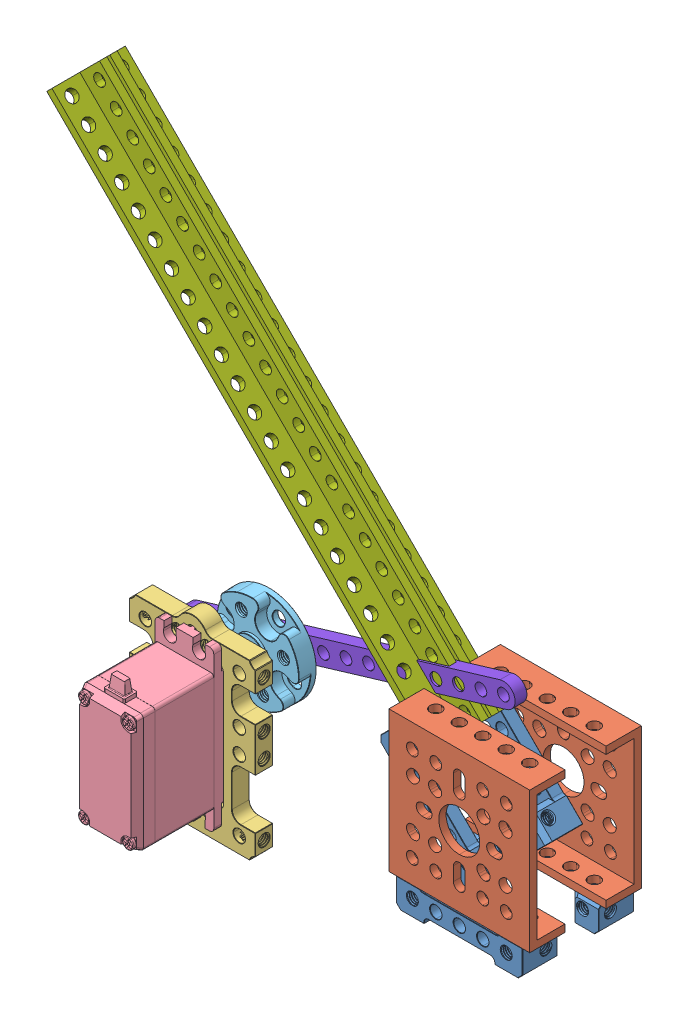
SolidWorks assembly League Meet 2 Drone Launcher Assembly, configuration Default. Lengths in mm.
Overall size (171.08 183.41 78.7).
24 component instances, 10 part files, 6 mates.
Components (placement in the parent):
- dual block.step-7: dual block.step [Default] at (-28.473 85.6625 -178.2749) x (0 1 0) z (0 0 -1) size (9.5 43 12)
- dual block.step-8: dual block.step [Default] at (-28.473 85.6625 -148.2749) x (0 1 0) z (0 0 1) size (9.5 43 12)
- 1 Hole Low-Side U Channel 48mm.step-1: 1 Hole Low-Side U Channel 48mm.step [Default] at (-52.473 119.1625 -158.2749) x (0 0 1) z (0 1 0) size (12 48 48)
- 1 Hole Low-Side U Channel 48mm.step-2: 1 Hole Low-Side U Channel 48mm.step [Default] at (-4.473 119.1625 -168.2749) x (0 0 -1) z (0 1 0) size (12 48 48)
- servomounts-1: servomounts [Default] at (-124.1137 126.6202 -137.5117) x (0 1 0) z (1 0 0) size (62.75 6.01 43)
  - 1802-0043-0001 assembly.STEP-1: 1802-0043-0001 assembly.STEP [Default] at origin size (72.97 22.74 55.08)
    - 1802-0043-0001.STEP-1: 1802-0043-0001.STEP [Default] at (-30.9577 -1.7632 15.6407) size (62.75 6.01 43)
    - 2800-0004-0010_90128A207.STEP-1: 2800-0004-0010_90128A207.STEP [Default] at (-69.1779 -7.2859 49.2191) size (7 7 14.01)
    - 2800-0004-0010_90128A207.STEP-2: 2800-0004-0010_90128A207.STEP [Default] at (-62.9116 -10.432 41.1189) size (7 7 14.01)
    - 2800-0004-0010_90128A207.STEP-3: 2800-0004-0010_90128A207.STEP [Default] at (-57.0244 -15.0047 35.4158) size (7 7 14.01)
    - 2800-0004-0010_90128A207.STEP-4: 2800-0004-0010_90128A207.STEP [Default] at (-43.2566 -10.2911 41.7146) size (7 7 14.01)
    - 2801-0004-0008_91166A230.STEP-1: 2801-0004-0008_91166A230.STEP [Default] at (-30.0387 -11.2295 43.9062) size (8 8 1)
    - 2801-0004-0008_91166A230.STEP-2: 2801-0004-0008_91166A230.STEP [Default] at (-23.3551 -8.712 41.3616) size (8 8 1)
    - 2801-0004-0008_91166A230.STEP-3: 2801-0004-0008_91166A230.STEP [Default] at (-15.3435 -8.8342 38.2183) size (8 8 1)
    - 2801-0004-0008_91166A230.STEP-4: 2801-0004-0008_91166A230.STEP [Default] at (-8.3583 -10.7984 34.7791) size (8 8 1)
- servo.step-6: servo.step [Default] at (-108.423 95.9125 -141.7749) x (0 -1 0) z (0 0 -1) size (54.3 20 43.9)
- 1910-0025-0816.STEP-1: 1910-0025-0816.STEP [Default] at (-84.4531 117.807 -167.0522) x (0.946981 0.321289 0) z (0.321289 -0.946981 0) size (32 17.1 32)
  - 1910-0025-0816.STEP-1: 1910-0025-0816.STEP [Default] at (-26.5689 7.4772 3.7047) size (32 15.6 32)
  - 2800-0003-0012.STEP-1: 2800-0003-0012.STEP [Default] at (-26.5689 24.5772 3.7047) x (0.895056 0 0.445953) z (0 1 0) size (5.5 5.5 15.01)
- dual block.step-9: dual block.step [Default] at (-28.473 108.9762 -175.7749) x (0.707107 0.707107 0) z (0 0 -1) size (9.5 43 12)
- dual block.step-10: dual block.step [Default] at (-28.473 108.9762 -150.7749) x (0.707107 0.707107 0) z (0 0 1) size (9.5 43 12)
- Lbeam.step-3: Lbeam.step [Default] at (-45.4436 108.9762 -163.7749) x (0.707107 0.707107 0) z (0 0 1) size (12 184 12)
- Lbeam.step-4: Lbeam.step [Default] at (-175.5512 239.0839 -162.7749) x (0.707107 0.707107 0) z (0 0 -1) size (12 184 12)
- 15 hole flat beam.step-1: 15 hole flat beam.step [Default] at (-82.382 113.9887 -163.5749) x (0.957945 0.286951 0) z (0.286951 -0.957945 0) size (120 4 8)
Mates (geometry in assembly coordinates):
- Parallel34: parallel aligned: plane of 1 Hole Low-Side U Channel 48mm.step-1 through (-4.473 119.1625 -179.7749) normal (0 0 1); plane of 1 Hole Low-Side U Channel 48mm.step-2 through (-52.473 73.6625 -144.2749) normal (0 0 1)
- Parallel37: parallel aligned: plane of 1 Hole Low-Side U Channel 48mm.step-2 through (-52.473 73.6625 -144.2749) normal (0 0 1); plane of Lbeam.step-3 through (-51.1004 114.6331 -163.7749) normal (0 0 1)
- Parallel38: parallel anti-aligned: plane of 1 Hole Low-Side U Channel 48mm.step-2 through (-52.473 73.6625 -144.2749) normal (0 0 1); plane of Lbeam.step-4 through (-169.8944 233.427 -162.7749) normal (0 0 -1)
- Coincident98: coincident anti-aligned: plane of 1910-0025-0816.STEP-1/1910-0025-0816.STEP-1 through (-108.423 105.7625 -159.5749) normal (0 0 -1); plane of 15 hole flat beam.step-1 through (-136.027 97.9194 -159.5749) normal (0 0 1)
- Tangent23: tangent: circle of Lbeam.step-3; plane of 15 hole flat beam.step-1 through (-137.1748 101.7512 -159.5749) normal (-0.286951 0.957945 0)
- Concentric68: concentric aligned: cylinder of 1910-0025-0816.STEP-1/1910-0025-0816.STEP-1; cylinder of 15 hole flat beam.step-1 through (-97.7092 109.3975 -159.5749) axis (0 0 1) radius 2
